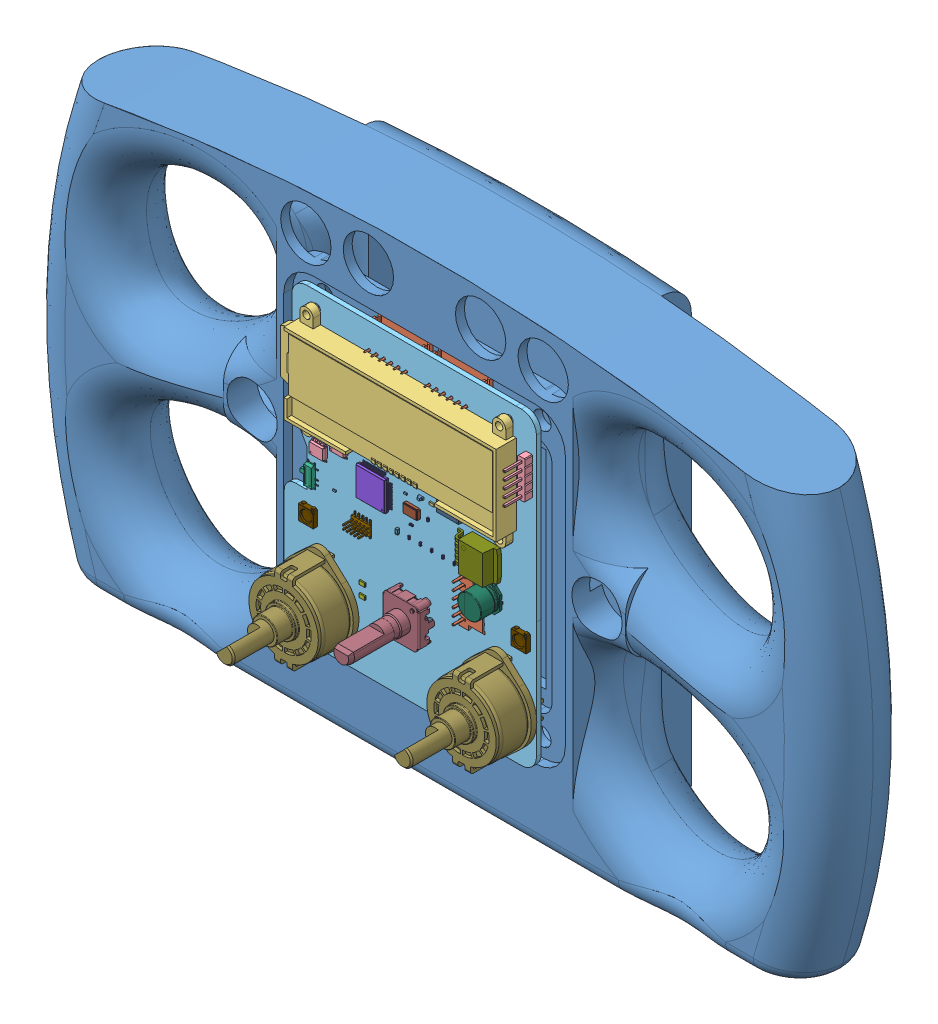
SolidWorks assembly Złożenie1, configuration Domyślna. Lengths in mm.
Overall size (272.81 155 79.14).
128 component instances, 24 part files, 0 mates.
Components (placement in the parent):
- kiera czesc glowna 11111-1: kiera czesc glowna 11111 [Domyślna] at origin size (272.81 155 46.22)
- Część1^Złożenie1-1: Część1^Złożenie1 [Domyślna] at origin (virtual)
- PGR-06_Wheel.step-2: PGR-06_Wheel.step [Domyślna] at (-112.7498 121.7452 32.8229) size (86.44 104.14 40.69)
  - 7447707331.step-1: 7447707331.step [Domyślna] at (134.62 -132.715 -0.05) x (0 1 0) z (0 0 -1) size (17.4 7.9 8.4)
    - COMPOUND.step-1: COMPOUND.step [Domyślna] at origin size (17.4 7.9 8.4)
  - NHD-C0220BiZ-FS_RGB-FBW-3VM.step-1: NHD-C0220BiZ-FS_RGB-FBW-3VM.step [Domyślna] at (77.584 -103.868 2.65) size (75.7 37.6 11)
    - COMPOUND-0.step-1: COMPOUND-0.step [Domyślna] at origin size (75.7 37.6 11)
  - 22-05-7065.step-1: 22-05-7065.step [Domyślna] at (104.775 -73.295 -2.49) x (-1 0 0) z (0 0 -1) size (17.4 7.9 8.4)
    - COMPOUND.step-1: COMPOUND.step [Domyślna] at origin size (17.4 7.9 8.4)
  - 22-05-7065.step-2: 22-05-7065.step [Domyślna] at (125.095 -73.295 -2.49) x (-1 0 0) z (0 0 -1) size (17.4 7.9 8.4)
    - COMPOUND.step-1: COMPOUND.step [Domyślna] at origin size (17.4 7.9 8.4)
  - PinHeader_1x05_P2.54mm_Vertical.step-1: PinHeader_1x05_P2.54mm_Vertical.step [Domyślna] at (152.4 -91.44 1.65) x (-1 0 0) z (0 0 1) size (2.54 12.7 11.54)
    - SOLID.step-1: SOLID.step [Domyślna] at origin size (2.54 12.7 11.54)
  - R_0402_1005Metric.step-1: R_0402_1005Metric.step [Domyślna] at (86.997 -123.698 1.65) size (1 0.5 0.35)
    - SOLID-1.step-1: SOLID-1.step [Domyślna] at origin size (1 0.5 0.35)
  - SW_SPDT_PCM12.step-1: SW_SPDT_PCM12.step [Domyślna] at (79.502 -122.936 1.65) x (0 -1 0) z (0 0 1) size (7.7 5 2)
    - SOLID-2.step-1: SOLID-2.step [Domyślna] at origin size (7.7 5 2)
  - R_0805_2012Metric.step-1: R_0805_2012Metric.step [Domyślna] at (119.126 -98.298 1.65) size (2 1.2 0.45)
    - SOLID-3.step-1: SOLID-3.step [Domyślna] at origin size (2 1.2 0.45)
  - LQFP-64_10x10mm_P0.5mm.step-1: LQFP-64_10x10mm_P0.5mm.step [Domyślna] at (100.345 -115.945 1.65) x (-1 0 0) z (0 0 1) size (12 12 1.5)
    - SOLID-4.step-1: SOLID-4.step [Domyślna] at origin size (12 12 1.5)
  - PinHeader_2x05_P1.27mm_Vertical_SMD.step-1: PinHeader_2x05_P1.27mm_Vertical_SMD.step [Domyślna] at (96.52 -128.905 1.65) x (0 1 0) z (0 0 1) size (5.57 6.35 4.4)
    - SOLID-5.step-1: SOLID-5.step [Domyślna] at origin size (5.57 6.35 4.4)
  - D_SMC.step-1: D_SMC.step [Domyślna] at (127.254 -107.696 1.65) x (-1 0 0) z (0 0 1) size (8 5.9 2.31)
    - SOLID-6.step-1: SOLID-6.step [Domyślna] at origin size (8 5.9 2.31)
  - ABM3B-16.000MHZ-10-1-U-T.step-1: ABM3B-16.000MHZ-10-1-U-T.step [Domyślna] at (113.284 -116.332 1.65) x (0 -1 0) z (-1 0 0) size (3.2 1.1 5)
    - COMPOUND-7.step-1: COMPOUND-7.step [Domyślna] at origin size (3.2 1.1 5)
  - Alpha_(Taiwan)_-_SR2512F-0110-19R0B-E9-N-W-159.step-1: Alpha_(Taiwan)_-_SR2512F-0110-19R0B-E9-N-W-159.step [Domyślna] at (143.792 -156.224 1.65) size (25 31 37.8)
    - COMPOUND-8.step-1: COMPOUND-8.step [Domyślna] at origin size (25 31 37.8)
  - Alpha_(Taiwan)_-_SR2512F-0110-19R0B-E9-N-W-159.step-2: Alpha_(Taiwan)_-_SR2512F-0110-19R0B-E9-N-W-159.step [Domyślna] at (83.792 -156.224 1.65) size (25 31 37.8)
    - COMPOUND-8.step-1: COMPOUND-8.step [Domyślna] at origin size (25 31 37.8)
  - R_0805_2012Metric.step-2: R_0805_2012Metric.step [Domyślna] at (96.52 -146.05 1.65) x (-1 0 0) z (0 0 1) size (2 1.2 0.45)
    - SOLID-3.step-1: SOLID-3.step [Domyślna] at origin size (2 1.2 0.45)
  - R_0805_2012Metric.step-3: R_0805_2012Metric.step [Domyślna] at (96.52 -149.86 1.65) x (-1 0 0) z (0 0 1) size (2 1.2 0.45)
    - SOLID-3.step-1: SOLID-3.step [Domyślna] at origin size (2 1.2 0.45)
  - EC12E-250.step-1: EC12E-250.step [Domyślna] at (113.792 -146.224 3.65) size (14 14.25 28.51)
    - SOLID-9.step-1: SOLID-9.step [Domyślna] at origin size (14 14.25 28.51)
  - C_0603_1608Metric.step-1: C_0603_1608Metric.step [Domyślna] at (111.506 -99.314 1.65) x (-1 0 0) z (0 0 1) size (1.6 0.8 0.8)
    - SOLID-10.step-1: SOLID-10.step [Domyślna] at origin size (1.6 0.8 0.8)
  - C_0603_1608Metric.step-2: C_0603_1608Metric.step [Domyślna] at (107.696 -99.314 1.65) x (-1 0 0) z (0 0 1) size (1.6 0.8 0.8)
    - SOLID-10.step-1: SOLID-10.step [Domyślna] at origin size (1.6 0.8 0.8)
  - R_0805_2012Metric.step-4: R_0805_2012Metric.step [Domyślna] at (84.328 -157.734 1.65) x (0 1 0) z (0 0 1) size (2 1.2 0.45)
    - SOLID-3.step-1: SOLID-3.step [Domyślna] at origin size (2 1.2 0.45)
  - R_0805_2012Metric.step-5: R_0805_2012Metric.step [Domyślna] at (84.328 -167.894 1.65) x (0 1 0) z (0 0 1) size (2 1.2 0.45)
    - SOLID-3.step-1: SOLID-3.step [Domyślna] at origin size (2 1.2 0.45)
  - R_0805_2012Metric.step-6: R_0805_2012Metric.step [Domyślna] at (90.043 -168.275 1.65) x (0 1 0) z (0 0 1) size (2 1.2 0.45)
    - SOLID-3.step-1: SOLID-3.step [Domyślna] at origin size (2 1.2 0.45)
  - R_0805_2012Metric.step-7: R_0805_2012Metric.step [Domyślna] at (119.126 -94.742 1.65) size (2 1.2 0.45)
    - SOLID-3.step-1: SOLID-3.step [Domyślna] at origin size (2 1.2 0.45)
  - 16SVPG330MX.step-1: 16SVPG330MX.step [Domyślna] at (139.192 -128.27 1.65) x (-1 0 0) z (0 1 0) size (9.01 7.1 8.31)
    - COMPOUND-11.step-1: COMPOUND-11.step [Domyślna] at origin size (9.01 7.1 8.31)
  - LM2575HVS-3.3_NOPB.step-1: LM2575HVS-3.3_NOPB.step [Domyślna] at (135.954 -117.602 1.65) x (-1 0 0) z (0 1 0) size (14.35 4.8 10.16)
    - COMPOUND-12.step-1: COMPOUND-12.step [Domyślna] at origin size (14.35 4.8 10.16)
  - 22-05-7065.step-3: 22-05-7065.step [Domyślna] at (141.875 -87.63 -2.49) x (0 -1 0) z (0 0 -1) size (17.4 7.9 8.4)
    - COMPOUND.step-1: COMPOUND.step [Domyślna] at origin size (17.4 7.9 8.4)
  - 22-05-7065.step-4: 22-05-7065.step [Domyślna] at (84.82 -87.63 -2.49) x (0 1 0) z (0 0 -1) size (17.4 7.9 8.4)
    - COMPOUND.step-1: COMPOUND.step [Domyślna] at origin size (17.4 7.9 8.4)
  - R_0805_2012Metric.step-8: R_0805_2012Metric.step [Domyślna] at (84.0505 -170.815 1.65) size (2 1.2 0.45)
    - SOLID-3.step-1: SOLID-3.step [Domyślna] at origin size (2 1.2 0.45)
  - R_0805_2012Metric.step-9: R_0805_2012Metric.step [Domyślna] at (78.613 -170.815 1.65) size (2 1.2 0.45)
    - SOLID-3.step-1: SOLID-3.step [Domyślna] at origin size (2 1.2 0.45)
  - R_0805_2012Metric.step-10: R_0805_2012Metric.step [Domyślna] at (79.5255 -160.655 1.65) size (2 1.2 0.45)
    - SOLID-3.step-1: SOLID-3.step [Domyślna] at origin size (2 1.2 0.45)
  - R_0805_2012Metric.step-11: R_0805_2012Metric.step [Domyślna] at (78.74 -157.226 1.65) size (2 1.2 0.45)
    - SOLID-3.step-1: SOLID-3.step [Domyślna] at origin size (2 1.2 0.45)
  - R_0805_2012Metric.step-12: R_0805_2012Metric.step [Domyślna] at (85.09 -153.67 1.65) x (0 -1 0) z (0 0 1) size (2 1.2 0.45)
    - SOLID-3.step-1: SOLID-3.step [Domyślna] at origin size (2 1.2 0.45)
  - R_0805_2012Metric.step-13: R_0805_2012Metric.step [Domyślna] at (83.82 -162.56 1.65) x (0 -1 0) z (0 0 1) size (2 1.2 0.45)
    - SOLID-3.step-1: SOLID-3.step [Domyślna] at origin size (2 1.2 0.45)
  - R_0805_2012Metric.step-14: R_0805_2012Metric.step [Domyślna] at (149.86 -154.432 1.65) x (0 1 0) z (0 0 1) size (2 1.2 0.45)
    - SOLID-3.step-1: SOLID-3.step [Domyślna] at origin size (2 1.2 0.45)
  - R_0805_2012Metric.step-15: R_0805_2012Metric.step [Domyślna] at (149.86 -159.512 1.65) x (0 1 0) z (0 0 1) size (2 1.2 0.45)
    - SOLID-3.step-1: SOLID-3.step [Domyślna] at origin size (2 1.2 0.45)
  - R_0805_2012Metric.step-16: R_0805_2012Metric.step [Domyślna] at (149.86 -165.862 1.65) x (0 1 0) z (0 0 1) size (2 1.2 0.45)
    - SOLID-3.step-1: SOLID-3.step [Domyślna] at origin size (2 1.2 0.45)
  - R_0805_2012Metric.step-17: R_0805_2012Metric.step [Domyślna] at (144.399 -170.307 1.65) size (2 1.2 0.45)
    - SOLID-3.step-1: SOLID-3.step [Domyślna] at origin size (2 1.2 0.45)
  - R_0805_2012Metric.step-18: R_0805_2012Metric.step [Domyślna] at (126.873 -167.767 1.65) size (2 1.2 0.45)
    - SOLID-3.step-1: SOLID-3.step [Domyślna] at origin size (2 1.2 0.45)
  - R_0805_2012Metric.step-19: R_0805_2012Metric.step [Domyślna] at (137.033 -169.291 1.65) size (2 1.2 0.45)
    - SOLID-3.step-1: SOLID-3.step [Domyślna] at origin size (2 1.2 0.45)
  - R_0805_2012Metric.step-20: R_0805_2012Metric.step [Domyślna] at (130.302 -170.688 1.65) x (0 -1 0) z (0 0 1) size (2 1.2 0.45)
    - SOLID-3.step-1: SOLID-3.step [Domyślna] at origin size (2 1.2 0.45)
  - R_0805_2012Metric.step-21: R_0805_2012Metric.step [Domyślna] at (130.302 -164.338 1.65) x (0 -1 0) z (0 0 1) size (2 1.2 0.45)
    - SOLID-3.step-1: SOLID-3.step [Domyślna] at origin size (2 1.2 0.45)
  - R_0805_2012Metric.step-22: R_0805_2012Metric.step [Domyślna] at (130.302 -157.988 1.65) x (0 -1 0) z (0 0 1) size (2 1.2 0.45)
    - SOLID-3.step-1: SOLID-3.step [Domyślna] at origin size (2 1.2 0.45)
  - C_0603_1608Metric.step-3: C_0603_1608Metric.step [Domyślna] at (97.536 -106.172 1.65) x (0 1 0) z (0 0 1) size (1.6 0.8 0.8)
    - SOLID-10.step-1: SOLID-10.step [Domyślna] at origin size (1.6 0.8 0.8)
  - C_0603_1608Metric.step-4: C_0603_1608Metric.step [Domyślna] at (108.458 -124.714 1.65) x (0 1 0) z (0 0 1) size (1.6 0.8 0.8)
    - SOLID-10.step-1: SOLID-10.step [Domyślna] at origin size (1.6 0.8 0.8)
  - C_0603_1608Metric.step-5: C_0603_1608Metric.step [Domyślna] at (94.996 -106.172 1.65) x (0 1 0) z (0 0 1) size (1.6 0.8 0.8)
    - SOLID-10.step-1: SOLID-10.step [Domyślna] at origin size (1.6 0.8 0.8)
  - C_0402_1005Metric.step-1: C_0402_1005Metric.step [Domyślna] at (112.268 -124.714 1.65) x (0 1 0) z (0 0 1) size (1 0.5 0.5)
    - SOLID-13.step-1: SOLID-13.step [Domyślna] at origin size (1 0.5 0.5)
  - C_0402_1005Metric.step-2: C_0402_1005Metric.step [Domyślna] at (116.078 -124.714 1.65) x (0 1 0) z (0 0 1) size (1 0.5 0.5)
    - SOLID-13.step-1: SOLID-13.step [Domyślna] at origin size (1 0.5 0.5)
  - C_0402_1005Metric.step-3: C_0402_1005Metric.step [Domyślna] at (119.888 -124.714 1.65) x (0 1 0) z (0 0 1) size (1 0.5 0.5)
    - SOLID-13.step-1: SOLID-13.step [Domyślna] at origin size (1 0.5 0.5)
  - C_0402_1005Metric.step-4: C_0402_1005Metric.step [Domyślna] at (123.698 -124.714 1.65) x (0 1 0) z (0 0 1) size (1 0.5 0.5)
    - SOLID-13.step-1: SOLID-13.step [Domyślna] at origin size (1 0.5 0.5)
  - C_0402_1005Metric.step-5: C_0402_1005Metric.step [Domyślna] at (127.508 -124.714 1.65) x (0 1 0) z (0 0 1) size (1 0.5 0.5)
    - SOLID-13.step-1: SOLID-13.step [Domyślna] at origin size (1 0.5 0.5)
  - C_0402_1005Metric.step-6: C_0402_1005Metric.step [Domyślna] at (114.935 -107.95 1.65) x (0 1 0) z (0 0 1) size (1 0.5 0.5)
    - SOLID-13.step-1: SOLID-13.step [Domyślna] at origin size (1 0.5 0.5)
  - C_0402_1005Metric.step-7: C_0402_1005Metric.step [Domyślna] at (113.03 -120.65 1.65) size (1 0.5 0.5)
    - SOLID-13.step-1: SOLID-13.step [Domyślna] at origin size (1 0.5 0.5)
  - C_0402_1005Metric.step-8: C_0402_1005Metric.step [Domyślna] at (111.76 -107.95 1.65) x (0 1 0) z (0 0 1) size (1 0.5 0.5)
    - SOLID-13.step-1: SOLID-13.step [Domyślna] at origin size (1 0.5 0.5)
  - C_0402_1005Metric.step-9: C_0402_1005Metric.step [Domyślna] at (118.618 -116.332 1.65) x (0 -1 0) z (0 0 1) size (1 0.5 0.5)
    - SOLID-13.step-1: SOLID-13.step [Domyślna] at origin size (1 0.5 0.5)
  - LED_WS2812B_PLCC4_5.0x5.0mm_P3.2mm.step-1: LED_WS2812B_PLCC4_5.0x5.0mm_P3.2mm.step [Domyślna] at (78.74 -134.62 1.65) x (0 1 0) z (0 0 1) size (5.4 5 1.6)
    - SOLID-14.step-1: SOLID-14.step [Domyślna] at origin size (5.4 5 1.6)
  - LED_WS2812B_PLCC4_5.0x5.0mm_P3.2mm.step-2: LED_WS2812B_PLCC4_5.0x5.0mm_P3.2mm.step [Domyślna] at (150.495 -135.255 1.65) x (0 1 0) z (0 0 1) size (5.4 5 1.6)
    - SOLID-14.step-1: SOLID-14.step [Domyślna] at origin size (5.4 5 1.6)
  - LED_0603_1608Metric.step-1: LED_0603_1608Metric.step [Domyślna] at (116.205 -111.125 1.65) x (-1 0 0) z (0 0 1) size (1.6 0.8 1.1)
    - SOLID-15.step-1: SOLID-15.step [Domyślna] at origin size (1.6 0.8 1.1)
  - L_0402_1005Metric.step-1: L_0402_1005Metric.step [Domyślna] at (108.585 -107.95 1.65) x (0 -1 0) z (0 0 1) size (1 0.5 0.5)
    - SOLID-16.step-1: SOLID-16.step [Domyślna] at origin size (1 0.5 0.5)
  - R_0603_1608Metric.step-1: R_0603_1608Metric.step [Domyślna] at (120.015 -111.125 1.65) x (-1 0 0) z (0 0 1) size (1.6 0.8 0.45)
    - SOLID-17.step-1: SOLID-17.step [Domyślna] at origin size (1.6 0.8 0.45)
  - R_0402_1005Metric.step-2: R_0402_1005Metric.step [Domyślna] at (110.998 -112.522 1.65) size (1 0.5 0.35)
    - SOLID-1.step-1: SOLID-1.step [Domyślna] at origin size (1 0.5 0.35)
  - SOIC-8_3.9x4.9mm_P1.27mm.step-1: SOIC-8_3.9x4.9mm_P1.27mm.step [Domyślna] at (82.296 -113.792 1.65) x (0 1 0) z (0 0 1) size (6 4.9 1.75)
    - SOLID-18.step-1: SOLID-18.step [Domyślna] at origin size (6 4.9 1.75)
  - SOIC-8_3.9x4.9mm_P1.27mm.step-2: SOIC-8_3.9x4.9mm_P1.27mm.step [Domyślna] at (89.154 -109.474 1.65) x (0 1 0) z (0 0 1) size (6 4.9 1.75)
    - SOLID-18.step-1: SOLID-18.step [Domyślna] at origin size (6 4.9 1.75)
  - COMPOUND-20.step-1: COMPOUND-20.step [Domyślna] at origin size (85.09 104.14 1.6)
